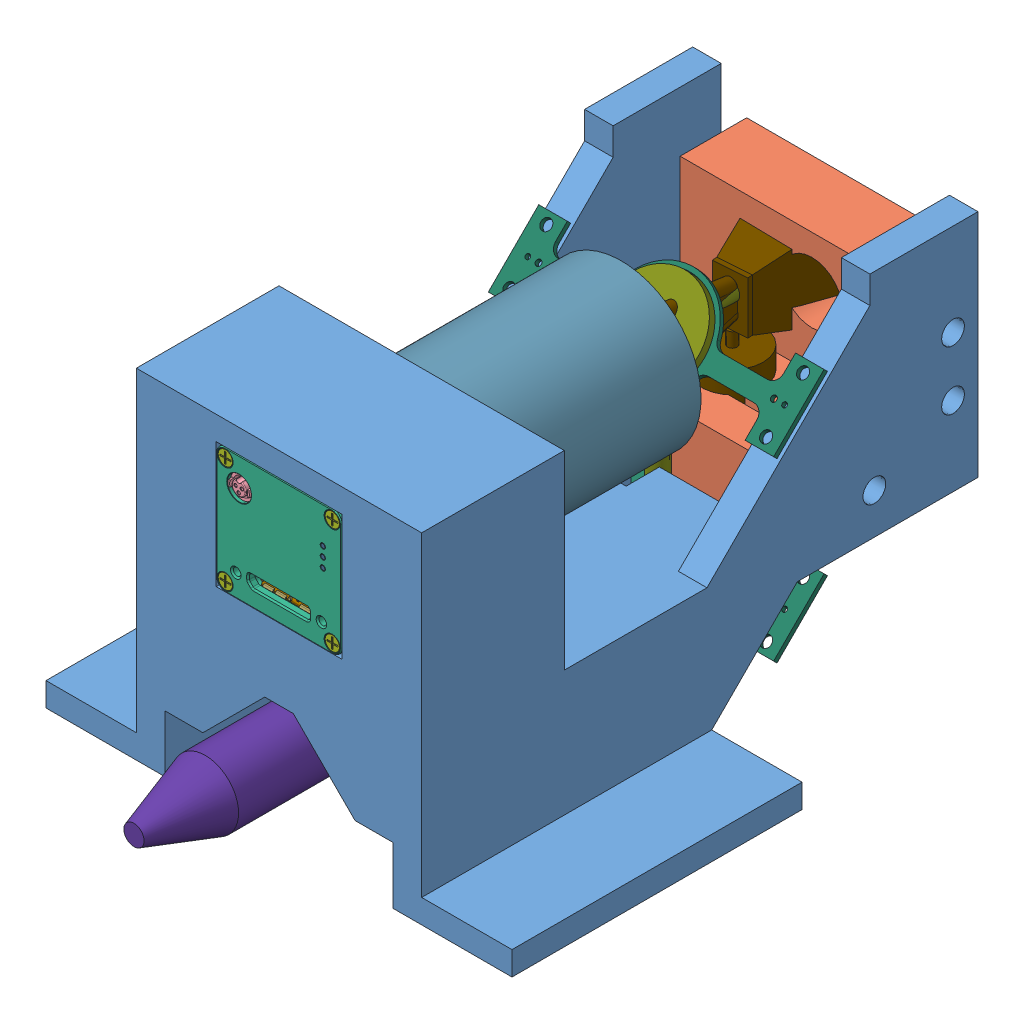
SolidWorks assembly Assem1, configuration Default. Lengths in mm.
Overall size (98 156.78 196.42).
54 component instances, 36 part files, 21 mates.
Components (placement in the parent):
- cam_holder_flip-1: cam_holder_flip [Default] at origin size (98 71.4 135.39)
- galvo_block-1: galvo_block [Default] at (-18.65 -27.87 0) x (0 -1 0) z (1 0 0) size (39.65 34.73 42.65)
- STP-MQ-(MQ022xG-CM)-ASSM-1: STP-MQ-(MQ022xG-CM)-ASSM [Default] at (0 -13.2 94.5) x (-1 0 0) z (0 0 -1) size (26.4 26.4 30.19)
  - STP-MQ-(MQ022xG-CM)-ASSM.stp-1: STP-MQ-(MQ022xG-CM)-ASSM.stp [Default] at origin size (26.4 26.4 30.19)
    - SUBASSM-MQ-FRONT.stp-1: SUBASSM-MQ-FRONT.stp [Default] x (0 -1 0) z (0 0 1) size (26.4 26.4 14.6)
      - MECH-MQ-FRONT.stp-1: MECH-MQ-FRONT.stp [Default] at (0 0 7.5) x (1 0 0) z (0 0 -1) size (26.4 26.4 7.5)
      - MECH-MQ-CS-C.stp-1: MECH-MQ-CS-C.stp [Default] at (0 0 0.5) x (1 0 0) z (0 0 -1) size (26.4 26.4 5.5)
      - SROB-M2x14-CUST.stp-1: SROB-M2x14-CUST.stp [Default] at (-11.25 11.25 -7.1) size (3 3 14.55)
      - SROB-M2x14-CUST.stp-2: SROB-M2x14-CUST.stp [Default] at (11.25 -11.25 -7.1) size (3 3 14.55)
      - SROB-M2x14-CUST.stp-3: SROB-M2x14-CUST.stp [Default] at (11.25 11.25 -7.1) size (3 3 14.55)
      - SROB-M2x14-CUST.stp-4: SROB-M2x14-CUST.stp [Default] at (-11.25 -11.25 -7.1) size (3 3 14.55)
    - SUBASSM-MQ-REAR.stp-1: SUBASSM-MQ-REAR.stp [Default] at (0 0 -22.584) x (-1 0 0) z (0 0 1) size (26.4 26.4 10.6)
      - MECH-MQ-REAR.stp-1: MECH-MQ-REAR.stp [Default] at (0 0 6.5) x (-1 0 0) z (0 0 -1) size (26.4 26.4 6.5)
      - SROB-M2x10-CUST .stp-1: SROB-M2x10-CUST .stp [Default] at (-11.25 11.25 10.6) x (1 0 0) z (0 0 -1) size (3 3 10.55)
      - SROB-M2x10-CUST .stp-2: SROB-M2x10-CUST .stp [Default] at (11.25 11.25 10.6) x (1 0 0) z (0 0 -1) size (3 3 10.55)
      - SROB-M2x10-CUST .stp-3: SROB-M2x10-CUST .stp [Default] at (11.25 -11.25 10.6) x (1 0 0) z (0 0 -1) size (3 3 10.55)
      - SROB-M2x10-CUST .stp-4: SROB-M2x10-CUST .stp [Default] at (-11.25 -11.25 10.6) x (1 0 0) z (0 0 -1) size (3 3 10.55)
      - MECH-MQ-THERMAL-PAD.stp-1: MECH-MQ-THERMAL-PAD.stp [Default] at (-10.5 5.45 4.8) x (0.961741 -0.273959 0) z (0 0 -1) size (20.28 8 0.5)
      - MECH-EMI-GSKT-1.3X2.3X11.stp-1: MECH-EMI-GSKT-1.3X2.3X11.stp [Default] at (0 9.9495 3.45) size (11 1.2 3)
      - MECH-EMI-GSKT-1.3X2.3X11.stp-2: MECH-EMI-GSKT-1.3X2.3X11.stp [Default] at (0 7.0505 3.45) size (11 1.2 3)
      - MECH-LIGHTPIPE-1.63X4.14.stp-1: MECH-LIGHTPIPE-1.63X4.14.stp [Default] at (9.3 -3.5 4.1492) x (-1 0 0) z (0 -1 0) size (1.63 4.14 1.63)
      - MECH-LIGHTPIPE-1.63X4.14.stp-2: MECH-LIGHTPIPE-1.63X4.14.stp [Default] at (9.3 -1.5 4.1492) x (-1 0 0) z (0 -1 0) size (1.63 4.14 1.63)
      - MECH-LIGHTPIPE-1.63X4.14.stp-3: MECH-LIGHTPIPE-1.63X4.14.stp [Default] at (9.3 -5.5 4.1492) x (-1 0 0) z (0 -1 0) size (1.63 4.14 1.63)
    - SUBASSM-MQ-MID-022-CM.stp-1: SUBASSM-MQ-MID-022-CM.stp [Default] at (0 0 -4.5) x (-1 0 0) z (0 0 -1) size (26.4 26.4 11.68)
      - MECH-MQ-MID-022-CM-REV2.stp-1: MECH-MQ-MID-022-CM-REV2.stp [Default] at origin size (26.4 26.4 11.59)
      - MECH-O-RING-22X1-VI370.stp-1: MECH-O-RING-22X1-VI370.stp [Default] at (0 0 1.3) x (1 0 0) z (0 1 0) size (24 1 24)
      - FLT-BK7-AR2X-D25.stp-1: FLT-BK7-AR2X-D25.stp [Default] at (0 0 -0.1) size (25 25 1.1)
      - MECH-MX022xG-CM-GSKT.stp-1: MECH-MX022xG-CM-GSKT.stp [Default] at (0 0 3.364) x (0 -1 0) z (0 0 1) size (12.2 17.4 1.27)
    - MQ022xG-CM-PCA-LW_MODEL.stp-1: MQ022xG-CM-PCA-LW_MODEL.stp [Default] at (0 0 -16.486) x (-1 0 0) z (0 0 -1) size (25.43 25.43 13.85)
      - CMV2000.stp-1: CMV2000.stp [Default] at (-0.0259 -0.5261 -1.002) x (-1 0 0) z (0 0 -1) size (18.65 13.5 6.65)
        - ANDON-96UPGA-Socket.stp-1: ANDON-96UPGA-Socket.stp [Default] at origin size (15.9 10.8 3.23)
        - CMV2000_Package.stp-1: CMV2000_Package.stp [Default] at (0 0 3.29) x (-1 0 0) z (0 0 1) size (18.65 13.5 5.45)
        - CMV2000_Glass.stp-1: CMV2000_Glass.stp [Default] at (0 0 6.1) size (18.06 12.95 0.55)
      - MQ022xG-CM-PCA-LW_MODEL-0.stp-1: MQ022xG-CM-PCA-LW_MODEL-0.stp [Default] at origin size (0.25 1.57 4.1)
      - MQ022xG-CM-PCA-LW_MODEL-1.stp-1: MQ022xG-CM-PCA-LW_MODEL-1.stp [Default] at origin size (12.85 2.05 3.8)
      - MQ022xG-CM-PCA-LW_MODEL-2.stp-1: MQ022xG-CM-PCA-LW_MODEL-2.stp [Default] at origin size (25.43 25.43 1)
      - MQ022xG-CM-PCA-LW_MODEL-3.stp-1: MQ022xG-CM-PCA-LW_MODEL-3.stp [Default] at origin size (0.25 1.57 4.1)
      - MQ022xG-CM-PCA-LW_MODEL-4.stp-1: MQ022xG-CM-PCA-LW_MODEL-4.stp [Default] at origin size (5 5 8.1)
      - MQ022xG-CM-PCA-LW_MODEL-5.stp-1: MQ022xG-CM-PCA-LW_MODEL-5.stp [Default] at origin size (0.25 1.57 4.1)
      - MQ022xG-CM-PCA-LW_MODEL-6.stp-1: MQ022xG-CM-PCA-LW_MODEL-6.stp [Default] at origin size (0.25 1.57 4.1)
      - MQ022xG-CM-PCA-LW_MODEL-7.stp-1: MQ022xG-CM-PCA-LW_MODEL-7.stp [Default] at origin size (0.25 1.57 4.1)
      - MQ022xG-CM-PCA-LW_MODEL-8.stp-1: MQ022xG-CM-PCA-LW_MODEL-8.stp [Default] at origin size (0.25 1.57 4.1)
      - MQ022xG-CM-PCA-LW_MODEL-9.stp-1: MQ022xG-CM-PCA-LW_MODEL-9.stp [Default] at origin size (0.25 1.57 4.1)
      - MQ022xG-CM-PCA-LW_MODEL-10.stp-1: MQ022xG-CM-PCA-LW_MODEL-10.stp [Default] at origin size (0.25 1.57 4.1)
      - MQ022xG-CM-PCA-LW_MODEL-11.stp-1: MQ022xG-CM-PCA-LW_MODEL-11.stp [Default] at origin size (0.25 1.57 4.1)
      - MQ022xG-CM-PCA-LW_MODEL-12.stp-1: MQ022xG-CM-PCA-LW_MODEL-12.stp [Default] at origin size (13.8 3 5.6)
      - MQ022xG-CM-PCA-LW_MODEL-13.stp-1: MQ022xG-CM-PCA-LW_MODEL-13.stp [Default] at origin size (0.25 1.57 4.1)
- lens-1: lens [Default] at (0 -13.2 45) x (-0.538752 0.842464 0) z (0 0 1) size (33.5 33.5 46.47)
- D_holder-1: D_holder [Default] at (0 -13.5536 36.9678) x (1 0 0) z (0 0.707107 0.707107) size (60 22 1)
- mirror-1: mirror [Default] at (0 -13.2 37.3213) x (1 0 0) z (0 0.707107 0.707107) size (20 121.63 78.36)
- D_holder-2: D_holder [Default] at (0 -50.0673 37.6749) x (1 0 0) z (0 -0.707107 -0.707107) size (60 22 1)
- mirror-2: mirror [Default] at (0 -50.4208 37.3213) x (-1 0 0) z (0 -0.707107 -0.707107) size (20 121.63 78.36)
- laser-1: laser [Default] at (0.2271 -49.5462 51.7323) size (14 14 96)
- glavo-1: glavo [Default] at (0.075 -60.2656 21.745) x (-0.997449 0 0.071383) z (-0.071383 0 -0.997449) size (26 59.2 96.5)
Mates (geometry in assembly coordinates):
- Concentric1: concentric aligned: cylinder of cam_holder_flip-1 through (-30 -14.37 5.25) axis (-1 0 0) radius 2.4; cylinder of galvo_block-1 through (-18.65 -14.37 5.25) axis (-1 0 0) radius 1.25
- Concentric2: concentric aligned: cylinder of cam_holder_flip-1 through (-30 -34.86 21.8) axis (-1 0 0) radius 2.4; cylinder of galvo_block-1 through (-18.65 -34.86 21.8) axis (-1 0 0) radius 1.25
- Coincident3: coincident anti-aligned: plane of cam_holder_flip-1 through (13.2 0 117) normal (-1 0 0); plane of STP-MQ-(MQ022xG-CM)-ASSM-1/STP-MQ-(MQ022xG-CM)-ASSM.stp-1/SUBASSM-MQ-FRONT.stp-1/MECH-MQ-FRONT.stp-1 through (13.2 -26.4 94.5) normal (1 0 0)
- Coincident4: coincident anti-aligned: plane of cam_holder_flip-1 through (-13.2 -26.4 117) normal (0 1 0); plane of STP-MQ-(MQ022xG-CM)-ASSM-1/STP-MQ-(MQ022xG-CM)-ASSM.stp-1/SUBASSM-MQ-FRONT.stp-1/MECH-MQ-FRONT.stp-1 through (-13.2 -26.4 94.5) normal (0 -1 0)
- Coincident5: coincident aligned: plane of cam_holder_flip-1 through (0 0 87) normal (0 0 -1); plane of STP-MQ-(MQ022xG-CM)-ASSM-1/STP-MQ-(MQ022xG-CM)-ASSM.stp-1/SUBASSM-MQ-FRONT.stp-1/MECH-MQ-FRONT.stp-1 through (-13.2 0 87) normal (0 0 -1)
- Concentric3: concentric aligned: cylinder of STP-MQ-(MQ022xG-CM)-ASSM-1/STP-MQ-(MQ022xG-CM)-ASSM.stp-1/SUBASSM-MQ-FRONT.stp-1/MECH-MQ-FRONT.stp-1 through (0 -13.2 93.5) axis (0 0 -1) radius 12.2703; cylinder of lens-1 through (0 -13.2 91.47) axis (0 0 -1) radius 12.65
- Coincident6: coincident anti-aligned: plane of cam_holder_flip-1 through (0 0 87) normal (0 0 -1); plane of lens-1 through (0 -13.2 87) normal (0 0 1)
- Coincident7: coincident anti-aligned: plane of cam_holder_flip-1 through (24 -35 87) normal (-1 0 0); plane of galvo_block-1 through (24 -27.87 0) normal (1 0 0)
- Concentric4: concentric aligned: circle of D_holder-1; circle of mirror-1
- Concentric5: concentric anti-aligned: cylinder of lens-1 through (0 -13.2 87) axis (0 0 -1) radius 16.75; cylinder of mirror-1 through (0 -13.2 17.3213) axis (0 0 1) radius 2
- Coincident10: coincident anti-aligned: plane of D_holder-1 through (0 -13.2 37.3213) normal (0 0.707107 0.707107); plane of mirror-1 through (0 -13.2 37.3213) normal (0 -0.707107 -0.707107)
- Parallel2: parallel anti-aligned: plane of cam_holder_flip-1 through (49 -0.7333 22.7333) normal (0 0.707107 0.707107); plane of D_holder-1 through (0 -13.5536 36.9678) normal (0 -0.707107 -0.707107)
- Parallel3: parallel aligned: line of cam_holder_flip-1 through (-24 5 22.7333) axis (-1 0 0); line of D_holder-1 through (-24 -7.5431 32.3716) axis (-1 0 0)
- Parallel4: parallel anti-aligned: plane of cam_holder_flip-1 through (49 -43.4 38) normal (0 -0.707107 -0.707107); plane of D_holder-2 through (0 -50.0673 37.6749) normal (0 0.707107 0.707107)
- Concentric6: concentric aligned: circle of D_holder-2; circle of mirror-2
- Coincident14: coincident aligned: plane of D_holder-2 through (0 -50.4208 37.3213) normal (0 -0.707107 -0.707107); circle of mirror-2
- Concentric7: concentric anti-aligned: cylinder of mirror-1 through (0 -23.2 37.3213) axis (0 1 0) radius 2; cylinder of mirror-2 through (0 -30.4208 37.3213) axis (0 -1 0) radius 2
- Parallel5: parallel anti-aligned: line of cam_holder_flip-1 through (30 -43.4 38) axis (-1 0 0); line of D_holder-2 through (24 -45.4711 31.6645) axis (1 0 0)
- Coincident16: coincident aligned: line of cam_holder_flip-1 through (0 -50.4208 36.15) axis (0 0 1); line of mirror-2 through (0 -50.4208 37.3213) axis (0 0 1)
- Coincident17: coincident anti-aligned: plane of cam_holder_flip-1 through (0 11.7071 11.7071) normal (0 0.707107 0.707107); plane of D_holder-1 through (0 -13.5536 36.9678) normal (0 -0.707107 -0.707107)
- Concentric8: concentric anti-aligned: cylinder of galvo_block-1 through (0.075 -70.52 21.745) axis (0 1 0) radius 6.425; cylinder of glavo-1 through (0.075 -23.2656 21.745) axis (0 -1 0) radius 6.5
